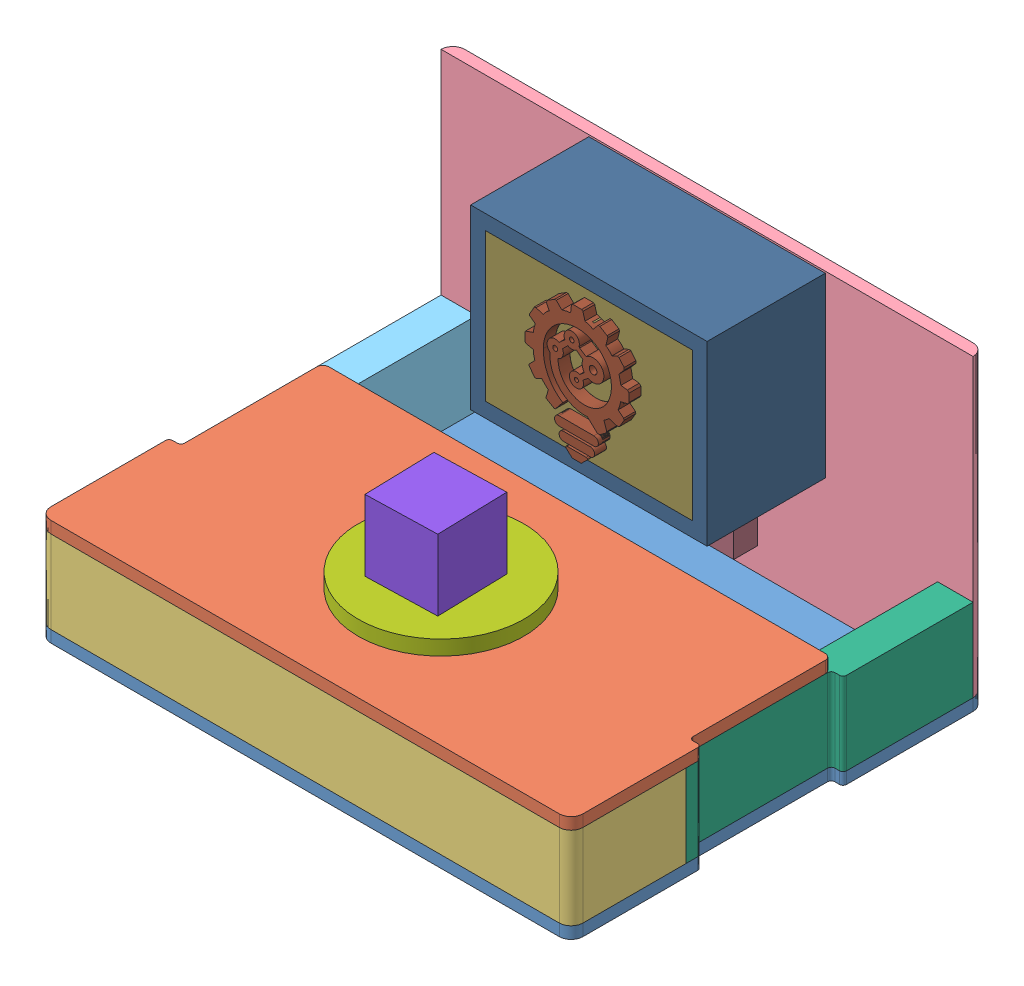
SolidWorks assembly Assem1, configuration Default. Lengths in mm.
Overall size (450 260 350).
29 component instances, 16 part files, 29 mates.
Components (placement in the parent):
- Part1-1: Part1 [Default] at (195.1879 217.8186 339.216) size (450 10 350)
- Part2-1: Part2 [Default] at (18.3581 297.8186 315.1445) size (450 10 230)
- Part3-1: Part3 [Default] at (225.5002 227.8186 429.8516) size (450 70 97)
- Part4-1: Part4 [Default] at (405.2273 227.8186 174.6875) x (-1 0 0) z (0 1 0) size (450 10 250)
- Part5-1: Part5 [Default] at (9.9515 227.8186 328.715) x (-1 0 0) z (0 0 -1) size (30 70 243)
- Part6-1: Part6 [Default] at (413.1247 227.8186 390.145) x (0 0 1) z (-1 0 0) size (243 70 30)
- Part9-1: Part9 [Default] at (195.1879 307.8186 399.216) x (0.074521 0 0.997219) z (-0.997219 0 0.074521) size (140 12.5 140)
- Part8-3: Part8 [Default] at (171.7481 320.3186 378.384) x (0.999639 0 -0.026875) z (0.026875 0 0.999639) size (60 60 60)
- ArduinoUno complet-1: ArduinoUno complet [Défaut] at (114.0463 227.8186 376.6323) x (0.012631 0 -0.99992) z (0.99992 0 0.012631) size (76.34 15.58 53.34)
- Part15-2: Part15 [Default] at (206.3562 418.9411 274.216) x (-1 0 0) z (0 0 -1) size (200 150 100)
- Part10-4: Part10 [Default] at (143.369 319.191 274.216) size (87.89 112.9 10)
- Part10 - Copie-2: Part10 - Copie [Default] at (143.369 319.191 270.716) size (175 125 16.52)
- Part7-1: Part7 [Default] at (207.4109 247.8218 171.9401) x (-1 0 0) z (0 0 -1) size (85 78.5 20)
- IR Sensor-1: IR Sensor [Default] at (228.2986 227.1374 356.7181) x (-1 0 0) z (0 1 0) size (30.59 30.6 76.32)
  - IR Sensor-1: IR Sensor [Default] at (33.1107 42.4979 39.3395) size (17.13 19.78 76.32)
  - Nut-1: Nut [Default] at (33.1107 42.4979 88.6964) x (0.695703 0.718329 0) z (0 0 -1) size (21.92 21.35 8.6)
- RED LED-1: RED LED [Default] at (222.4486 363.7003 255.734) size (4 16 4)
- RED LED-2: RED LED [Default] at (168.8858 364.7747 254.0288) size (4 16 4)
- RED LED-3: RED LED [Default] at (216.1101 351.3361 256.2046) size (4 16 4)
- RED LED-4: RED LED [Default] at (175.0016 350.7107 254.9036) size (4 16 4)
- RED LED-5: RED LED [Default] at (147.2415 399.7424 254.1978) size (4 16 4)
- RED LED-6: RED LED [Default] at (150.0518 433.0531 254.6628) size (4 16 4)
- RED LED-7: RED LED [Default] at (242.5548 395.8687 255.903) size (4 16 4)
- RED LED-8: RED LED [Default] at (244.7103 429.3566 257.3972) size (4 16 4)
- RED LED-9: RED LED [Default] at (207.5901 399.9056 256.577) size (4 16 4)
- RED LED-10: RED LED [Default] at (162.0815 452.7714 253.8646) size (4 16 4)
- RED LED-11: RED LED [Default] at (230.2413 451.8864 255.9408) size (4 16 4)
- RED LED-12: RED LED [Default] at (188.2754 415.4546 254.8391) size (4 16 4)
- RED LED-13: RED LED [Default] at (204.2069 433.8975 255.8608) x (0.994994 0.044221 -0.089618) z (0.089412 0.006613 0.995973) size (4 16 4)
Mates (geometry in assembly coordinates):
- Coincident1: coincident anti-aligned: plane of Part1-1 through (195.1879 227.8186 339.216) normal (0 1 0); plane of Part3-1 through (225.5002 227.8186 429.8516) normal (0 -1 0)
- Concentric1: concentric aligned: cylinder of Part1-1 through (410.1879 227.8186 504.216) axis (0 -1 0) radius 10; cylinder of Part3-1 through (410.1879 297.8186 504.216) axis (0 -1 0) radius 10
- Coincident2: coincident anti-aligned: plane of Part2-1 through (18.3581 297.8186 315.1445) normal (0 -1 0); plane of Part3-1 through (225.5002 297.8186 429.8516) normal (0 1 0)
- Coincident4: coincident anti-aligned: circle of Part2-1; circle of Part3-1
- Coincident5: coincident anti-aligned: plane of Part1-1 through (195.1879 227.8186 339.216) normal (0 1 0); plane of Part4-1 through (405.2273 227.8186 174.6875) normal (0 -1 0)
- Coincident6: coincident aligned: plane of Part1-1 through (-29.8121 227.8186 164.216) normal (0 0 -1); plane of Part4-1 through (-29.8121 477.8186 164.216) normal (0 0 -1)
- Concentric2: concentric aligned: cylinder of Part1-1 through (410.1879 227.8186 174.216) axis (0 -1 0) radius 10; cylinder of Part4-1 through (410.1879 477.8186 174.216) axis (0 -1 0) radius 10
- Coincident7: coincident anti-aligned: plane of Part3-1 through (-29.8121 297.8186 417.216) normal (0 0 -1); plane of Part6-1 through (420.1879 297.8186 417.216) normal (0 0 1)
- Coincident8: coincident aligned: plane of Part1-1 through (410.1879 217.8186 404.216) normal (1 0 0); plane of Part6-1 through (410.1879 227.8186 404.216) normal (1 0 0)
- Coincident9: coincident anti-aligned: plane of Part4-1 through (-29.8121 477.8186 174.216) normal (0 0 1); plane of Part6-1 through (420.1879 297.8186 174.216) normal (0 0 -1)
- Coincident10: coincident anti-aligned: plane of Part2-1 through (18.3581 297.8186 315.1445) normal (0 -1 0); plane of Part6-1 through (413.1247 297.8186 390.145) normal (0 1 0)
- Coincident11: coincident anti-aligned: plane of Part1-1 through (195.1879 227.8186 339.216) normal (0 1 0); plane of Part5-1 through (9.9515 227.8186 328.715) normal (0 -1 0)
- Coincident12: coincident anti-aligned: plane of Part3-1 through (-29.8121 297.8186 417.216) normal (0 0 -1); plane of Part5-1 through (0.1879 297.8186 417.216) normal (0 0 1)
- Coincident13: coincident aligned: plane of Part1-1 through (-29.8121 227.8186 514.216) normal (-1 0 0); plane of Part5-1 through (-29.8121 297.8186 417.216) normal (-1 0 0)
- Concentric3: concentric aligned: circle of Part2-1; cylinder of Part9-1 through (195.1879 310.3186 399.216) axis (0 1 0) radius 11
- Coincident16: coincident anti-aligned: plane of Part2-1 through (18.3581 307.8186 315.1445) normal (0 1 0); plane of Part9-1 through (195.1879 307.8186 399.216) normal (0 -1 0)
- Coincident17: coincident anti-aligned: plane of Part9-1 through (195.1879 320.3186 399.216) normal (0 1 0); plane of Part8-3 through (171.7481 320.3186 378.384) normal (0 -1 0)
- Coincident22: coincident anti-aligned: plane of Part1-1 through (195.1879 227.8186 339.216) normal (0 1 0); plane of ArduinoUno complet-1 through (114.0463 227.8186 376.6323) normal (0 -1 0)
- Coincident32: coincident anti-aligned: line of Part15-2 through (282.6911 463.8218 274.216) axis (-1 0 0); line of Part10 - Copie-2 through (107.6911 463.8218 274.216) axis (1 0 0)
- Coincident33: coincident anti-aligned: line of Part15-2 through (107.6911 463.8218 274.216) axis (0 -1 0); line of Part10 - Copie-2 through (107.6911 338.8218 274.216) axis (0 1 0)
- Coincident34: coincident anti-aligned: line of Part10-4 through (199.0858 456.7347 274.216) axis (-1 0 0); line of Part10 - Copie-2 through (191.574 456.7347 274.216) axis (1 0 0)
- Coincident35: coincident: point of Part10-4; moEndPointRef_w of Part10 - Copie-2
- Coincident37: coincident aligned: line of Part2-1 through (-29.8121 297.8186 407.216) axis (0 0 1); line of Part3-1 through (-29.8121 297.8186 417.216) axis (0 0 1)
- Coincident44: coincident anti-aligned: circle of Part4-1; circle of Part15-2
- Parallel2: parallel aligned: line of Part4-1 through (-29.8121 477.8186 174.216) axis (1 0 0); line of Part15-2 through (95.1911 476.3218 174.216) axis (1 0 0)
- Coincident45: coincident anti-aligned: plane of Part15-2 through (295.1911 326.3218 174.216) normal (0 -1 0); plane of Part7-1 through (207.4109 326.3218 171.9401) normal (0 1 0)
- Coincident46: coincident aligned: line of Part15-2 through (157.6911 326.3218 184.216) axis (1 0 0); line of Part7-1 through (157.6911 326.3218 184.216) axis (1 0 0)
- Coincident47: coincident aligned: line of Part15-2 through (232.6911 326.3218 184.216) axis (0 0 -1); line of Part7-1 through (232.6911 326.3218 184.216) axis (0 0 -1)
- Concentric7: concentric anti-aligned: circle of Part2-1; circle of IR Sensor-1/Nut-1
